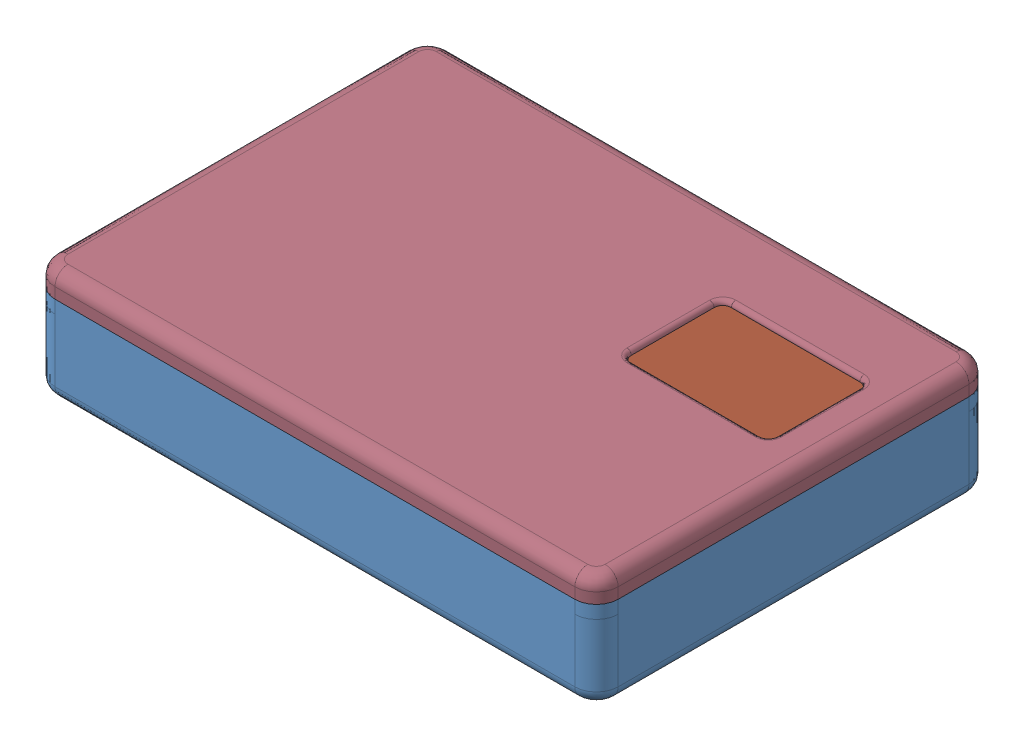
SolidWorks assembly Assembly, configuration Default. Lengths in mm. (continued)
Components (placement in the parent): (continued)
- PCB1_2.step-5: PCB1_2.step [Default] at (-142.0534 45.002 144.8645) x (1 0 -0.000465) z (0 1 0) size (68.54 35.94 11.54) (continued)
  - C21.step-1: C21.step [Default] at origin size (2 1.25 1.4) (continued)
    - Cap_Murata_GRM21BC81C106KA73L_eec.step-1: Cap_Murata_GRM21BC81C106KA73L_eec.step [Default] at (102.7788 62.357 0) x (-1 0 0) z (0 0 1) size (2 1.25 1.4) (continued)
      - 2-41.step-1: 2-41.step [Default] at (0 0 0.01) size (1.98 1.23 1.38)
      - Murata Logo 3.step-1: Murata Logo 3.step [Default] at (-0.1814 -0.5957 1.2901) size (0.53 0.12 0.1)
  - C20.step-1: C20.step [Default] at origin size (2 1.25 1.4)
    - Cap_Murata_GRM21BC81C106KA73L_eec.step-1: Cap_Murata_GRM21BC81C106KA73L_eec.step [Default] at (102.743 59.944 0) x (-1 0 0) z (0 0 1) size (2 1.25 1.4)
      - 1-40.step-1: 1-40.step [Default] at origin size (2 1.25 1.4)
      - 2-41.step-1: 2-41.step [Default] at (0 0 0.01) size (1.98 1.23 1.38)
      - Murata Logo 3.step-1: Murata Logo 3.step [Default] at (-0.1814 -0.5957 1.2901) size (0.53 0.12 0.1)
  - C19.step-1: C19.step [Default] at origin size (0.5 1 0.55)
    - Cap_Murata_GRM1552C1H271GA01J_eec.step-1: Cap_Murata_GRM1552C1H271GA01J_eec.step [Default] at (104.013 57.404 0) x (0 -1 0) z (0 0 1) size (1 0.5 0.55)
      - body-42.step-1: body-42.step [Default] x (-1 0 0) z (0 0 1) size (0.5 0.5 0.55)
      - side-43.step-1: side-43.step [Default] at (-0.2 0.6417 0) x (-1 0 0) z (0 0 1) size (0.25 0.5 0.55)
      - side-43.step-2: side-43.step [Default] at (0.2 0.6417 0.55) x (1 0 0) z (0 0 -1) size (0.25 0.5 0.55)
      - Murata-44.step-1: Murata-44.step [Default] at (-0.859 -0.6449 0.497) size (0.3 0.07 0.02)
  - C18.step-1: C18.step [Default] at origin size (0.8 1.6 0.87)
    - Cap_Wurth_885012206071_eec.step-1: Cap_Wurth_885012206071_eec.step [Default] at (112.903 54.737 0) x (0 -1 0) z (0 0 1) size (1.6 0.8 0.87)
      - terminals.step-1: terminals.step [Default] at origin size (1.6 0.8 0.87)
      - body-45.step-1: body-45.step [Default] at origin size (0.8 0.8 0.87)
      - logo.step-1: logo.step [Default] at (0 0.375 0.87) size (0.36 0.18 0)
  - C17.step-1: C17.step [Default] at origin size (1.25 2 1.4)
    - Cap_Murata_GRM21BC81C106KA73L_eec.step-1: Cap_Murata_GRM21BC81C106KA73L_eec.step [Default] at (90.297 60.071 0) x (0 1 0) z (0 0 1) size (2 1.25 1.4)
      - 1-40.step-1: 1-40.step [Default] at origin size (2 1.25 1.4)
      - 2-41.step-1: 2-41.step [Default] at (0 0 0.01) size (1.98 1.23 1.38)
      - Murata Logo 3.step-1: Murata Logo 3.step [Default] at (-0.1814 -0.5957 1.2901) size (0.53 0.12 0.1)
  - C16.step-1: C16.step [Default] at origin size (1.25 2 1.4)
    - Cap_Murata_GRM21BC81C106KA73L_eec.step-1: Cap_Murata_GRM21BC81C106KA73L_eec.step [Default] at (87.503 60.071 0) x (0 1 0) z (0 0 1) size (2 1.25 1.4)
      - 1-40.step-1: 1-40.step [Default] at origin size (2 1.25 1.4)
      - 2-41.step-1: 2-41.step [Default] at (0 0 0.01) size (1.98 1.23 1.38)
      - Murata Logo 3.step-1: Murata Logo 3.step [Default] at (-0.1814 -0.5957 1.2901) size (0.53 0.12 0.1)
  - C14.step-1: C14.step [Default] at origin size (1.6 0.8 0.87)
    - Cap_Wurth_885012206071_eec.step-1: Cap_Wurth_885012206071_eec.step [Default] at (98.159 54.102 0) x (-1 0 0) z (0 0 1) size (1.6 0.8 0.87)
      - terminals.step-1: terminals.step [Default] at origin size (1.6 0.8 0.87)
      - body-45.step-1: body-45.step [Default] at origin size (0.8 0.8 0.87)
      - logo.step-1: logo.step [Default] at (0 0.375 0.87) size (0.36 0.18 0)
  - C13.step-1: C13.step [Default] at origin size (0.8 1.6 0.87)
    - Cap_Wurth_885012206071_eec.step-1: Cap_Wurth_885012206071_eec.step [Default] at (110.998 54.737 0) x (0 1 0) z (0 0 1) size (1.6 0.8 0.87)
      - terminals.step-1: terminals.step [Default] at origin size (1.6 0.8 0.87)
      - body-45.step-1: body-45.step [Default] at origin size (0.8 0.8 0.87)
      - logo.step-1: logo.step [Default] at (0 0.375 0.87) size (0.36 0.18 0)
  - C12.step-1: C12.step [Default] at origin size (0.8 1.6 0.87)
    - Cap_Wurth_885012206071_eec.step-1: Cap_Wurth_885012206071_eec.step [Default] at (109.22 54.737 0) x (0 1 0) z (0 0 1) size (1.6 0.8 0.87)
      - terminals.step-1: terminals.step [Default] at origin size (1.6 0.8 0.87)
      - body-45.step-1: body-45.step [Default] at origin size (0.8 0.8 0.87)
      - logo.step-1: logo.step [Default] at (0 0.375 0.87) size (0.36 0.18 0)
  - C11.step-1: C11.step [Default] at origin size (2 1.25 1.46)
    - Cap_Murata_GRM21BC71C106KE11L_eec.step-1: Cap_Murata_GRM21BC71C106KE11L_eec.step [Default] at (106.2358 62.357 0) x (-1 0 0) z (0 0 1) size (2 1.25 1.46)
      - body-30.step-1: body-30.step [Default] x (-1 0 0) z (0 0 1) size (1.1 1.25 1.45)
      - side.step-1: side.step [Default] at (-0.7 0.2667 0) x (-1 0 0) z (0 0 1) size (0.45 1.25 1.45)
      - side.step-2: side.step [Default] at (0.7 0.2667 1.45) x (1 0 0) z (0 0 -1) size (0.45 1.25 1.45)
      - Murata.step-1: Murata.step [Default] at (-0.7353 -0.8898 1.447) size (0.61 0.14 0.01)
  - C10.step-1: C10.step [Default] at origin size (2 1.25 1.46)
    - Cap_Murata_GRM21BC71C106KE11L_eec.step-1: Cap_Murata_GRM21BC71C106KE11L_eec.step [Default] at (106.2352 59.944 0) x (-1 0 0) z (0 0 1) size (2 1.25 1.46)
      - body-30.step-1: body-30.step [Default] x (-1 0 0) z (0 0 1) size (1.1 1.25 1.45)
      - side.step-1: side.step [Default] at (-0.7 0.2667 0) x (-1 0 0) z (0 0 1) size (0.45 1.25 1.45)
      - side.step-2: side.step [Default] at (0.7 0.2667 1.45) x (1 0 0) z (0 0 -1) size (0.45 1.25 1.45)
      - Murata.step-1: Murata.step [Default] at (-0.7353 -0.8898 1.447) size (0.61 0.14 0.01)
  - C9.step-1: C9.step [Default] at origin size (0.5 1 0.55)
    - Cap_Murata_GRM1552C1H271GA01J_eec.step-1: Cap_Murata_GRM1552C1H271GA01J_eec.step [Default] at (105.791 57.404 0) x (0 1 0) z (0 0 1) size (1 0.5 0.55)
      - body-42.step-1: body-42.step [Default] x (-1 0 0) z (0 0 1) size (0.5 0.5 0.55)
      - side-43.step-1: side-43.step [Default] at (-0.2 0.6417 0) x (-1 0 0) z (0 0 1) size (0.25 0.5 0.55)
      - side-43.step-2: side-43.step [Default] at (0.2 0.6417 0.55) x (1 0 0) z (0 0 -1) size (0.25 0.5 0.55)
      - Murata-44.step-1: Murata-44.step [Default] at (-0.859 -0.6449 0.497) size (0.3 0.07 0.02)
  - C8.step-1: C8.step [Default] at origin size (0.8 1.6 0.87)
    - Cap_Wurth_885012206071_eec.step-1: Cap_Wurth_885012206071_eec.step [Default] at (118.237 59.309 0) x (0 1 0) z (0 0 1) size (1.6 0.8 0.87)
      - terminals.step-1: terminals.step [Default] at origin size (1.6 0.8 0.87)
      - body-45.step-1: body-45.step [Default] at origin size (0.8 0.8 0.87)
      - logo.step-1: logo.step [Default] at (0 0.375 0.87) size (0.36 0.18 0)
  - C7.step-1: C7.step [Default] at origin size (0.8 1.6 0.87)
    - Cap_Wurth_885012206071_eec.step-1: Cap_Wurth_885012206071_eec.step [Default] at (109.728 59.182 0) x (0 1 0) z (0 0 1) size (1.6 0.8 0.87)
      - terminals.step-1: terminals.step [Default] at origin size (1.6 0.8 0.87)
      - body-45.step-1: body-45.step [Default] at origin size (0.8 0.8 0.87)
      - logo.step-1: logo.step [Default] at (0 0.375 0.87) size (0.36 0.18 0)
  - C6.step-1: C6.step [Default] at origin size (0.9 1.7 0.9)
    - 6262525248.step-1: 6262525248.step [Default] at (74.295 49.53 -1.3104) size (0.9 1 0.9)
      - Extruded-46.step-1: Extruded-46.step [Default] at origin size (0.9 1 0.9)
    - 6262525088.step-1: 6262525088.step [Default] at (74.295 48.855 -1.3104) size (0.9 0.35 0.9)
      - Extruded-47.step-1: Extruded-47.step [Default] at origin size (0.9 0.35 0.9)
    - 6262525088.step-2: 6262525088.step [Default] at (74.295 50.205 -1.3104) size (0.9 0.35 0.9)
      - Extruded-47.step-1: Extruded-47.step [Default] at origin size (0.9 0.35 0.9)
  - C5.step-1: C5.step [Default] at origin size (0.9 1.7 0.9)
    - 6262525248.step-1: 6262525248.step [Default] at (74.295 52.959 -1.3104) size (0.9 1 0.9)
      - Extruded-46.step-1: Extruded-46.step [Default] at origin size (0.9 1 0.9)
    - 6262525088.step-1: 6262525088.step [Default] at (74.295 53.634 -1.3104) size (0.9 0.35 0.9)
      - Extruded-47.step-1: Extruded-47.step [Default] at origin size (0.9 0.35 0.9)
    - 6262525088.step-2: 6262525088.step [Default] at (74.295 52.284 -1.3104) size (0.9 0.35 0.9)
      - Extruded-47.step-1: Extruded-47.step [Default] at origin size (0.9 0.35 0.9)
  - C4.step-1: C4.step [Default] at origin size (1.25 2 1.45)
    - 6259391984.step-1: 6259391984.step [Default] at (85.471 49.217 0) x (0 -1 0) z (0 0 1) size (2 1.25 1.45)
      - Fillet1-48.step-1: Fillet1-48.step [Default] at origin size (0.45 1.25 1.45)
      - Fillet2-49.step-1: Fillet2-49.step [Default] at origin size (0.45 1.25 1.45)
      - body2-50.step-1: body2-50.step [Default] at origin size (1.1 1.22 1.42)
  - C3.step-1: C3.step [Default] at origin size (2 1.25 1.4)
    - Cap_Murata_GRM21BC81C106KA73L_eec.step-1: Cap_Murata_GRM21BC81C106KA73L_eec.step [Default] at (124.46 53.594 0) size (2 1.25 1.4)
      - 1-40.step-1: 1-40.step [Default] at origin size (2 1.25 1.4)
      - 2-41.step-1: 2-41.step [Default] at (0 0 0.01) size (1.98 1.23 1.38)
      - Murata Logo 3.step-1: Murata Logo 3.step [Default] at (-0.1814 -0.5957 1.2901) size (0.53 0.12 0.1)
  - C2.step-1: C2.step [Default] at origin size (1.25 2 1.4)
    - Cap_Murata_GRM21BC81C106KA73L_eec.step-1: Cap_Murata_GRM21BC81C106KA73L_eec.step [Default] at (121.285 53.213 0) x (0 1 0) z (0 0 1) size (2 1.25 1.4)
      - 1-40.step-1: 1-40.step [Default] at origin size (2 1.25 1.4)
      - 2-41.step-1: 2-41.step [Default] at (0 0 0.01) size (1.98 1.23 1.38)
      - Murata Logo 3.step-1: Murata Logo 3.step [Default] at (-0.1814 -0.5957 1.2901) size (0.53 0.12 0.1)
  - C1.step-1: C1.step [Default] at origin size (1.6 0.8 0.8)
    - 6259394864.step-1: 6259394864.step [Default] at (124.46 44.577 0.4) x (0 -1 0) z (-1 0 0) size (0.8 0.8 1.6)
- 18650 battery holder-1: 18650 battery holder [Výchozí] at (48.1858 46.5359 152.1637) x (0 0 1) z (-1 0 0) size (39.8 18.9 86.4)
  - 18650 baterie-1: 18650 baterie [Výchozí] at (-5.3689 1.7057 32.3879) size (18.5 18.5 64.78)
  - 18650 holder 2x-1: 18650 holder 2x [Výchozí] at (-14.7189 1.7057 25.8879) size (39.8 15.3 86.4)
  - 18650 baterie-2: 18650 baterie [Výchozí] at (-24.0689 1.7057 32.3879) size (18.5 18.5 64.78)
- ASSEMBLY_AP214.STEP-1: ASSEMBLY_AP214.STEP [Default] at (-14.6491 31.0882 66.6987) x (1 0 -0.000465) z (0.000465 0 1) size (17.79 12.75 33.03)
  - Crystal_Low_Profile.STEP-1: Crystal_Low_Profile.STEP [Default] at (9.717 16.7052 22.6754) x (0 0 -1) z (0 1 0) size (3.81 1.63 0.79)
    - Fusion001.STEP-1: Fusion001.STEP [Default] at origin size (3.81 1.63 0.79)
  - board.STEP-1: board.STEP [Default] at (5.4752 15.0552 41.6975) size (17.78 1.67 33.02)
  - ATmega.STEP-1: ATmega.STEP [Default] at (14.3652 16.8027 27.7275) x (0.707107 0 0.707107) z (-0.707107 0 0.707107) size (9 1.1 9)
  - cap_603.STEP-1: cap_603.STEP [Default] at (10.3417 16.7052 40.4401) x (0 0 -1) z (1 0 0) size (1.6 0.8 0.8)
  - cap_603.STEP-2: cap_603.STEP [Default] at (13.6922 16.7052 34.8585) size (1.6 0.8 0.8)
  - cap_603.STEP-3: cap_603.STEP [Default] at (11.8634 16.7052 21.6759) size (1.6 0.8 0.8)
  - cap_603.STEP-4: cap_603.STEP [Default] at (17.4768 16.7052 12.8875) size (1.6 0.8 0.8)
  - res_603.STEP-1: res_603.STEP [Default] at (10.4218 16.7052 37.2651) x (0 0 -1) z (1 0 0) size (1.6 0.5 0.8)
  - res_603.STEP-2: res_603.STEP [Default] at (19.5912 16.7052 37.5953) x (0 0 -1) z (1 0 0) size (1.6 0.5 0.8)
  - res_603.STEP-3: res_603.STEP [Default] at (15.1652 16.7052 14.6275) x (-1 0 0) z (0 0 -1) size (1.6 0.5 0.8)
  - condensateurTantale_106C_D_faut.STEP-1: condensateurTantale_106C_D_faut.STEP [Default] at (10.1742 17.5052 15.6625) x (0 0 -1) z (1 0 0) size (3.2 1.6 1.6)
  - condensateurTantale_106C_D_faut.STEP-2: condensateurTantale_106C_D_faut.STEP [Default] at (18.6832 17.5052 17.5675) x (0 0 -1) z (1 0 0) size (3.2 1.6 1.6)
  - SOT23-5.STEP-1: SOT23-5.STEP [Default] at (14.3653 16.6848 17.5167) x (1 0 0) z (0 1 0) size (2.84 3 1.19)
  - Surface Mount Chip LED 3.2x1.6mm.STEP-1: Surface Mount Chip LED 3.2x1.6mm.STEP [Default] at (18.7112 16.7112 39.0103) x (0 0 1) z (0 1 0) size (1.92 0.96 0.79)
  - Surface Mount Chip LED 3.2x1.6mm.STEP-2: Surface Mount Chip LED 3.2x1.6mm.STEP [Default] at (13.4306 16.7112 20.3081) x (1 0 0) z (0 1 0) size (1.92 0.96 0.79)
  - TACTILE-SWITCH-SMD-ALT01.STEP-1: TACTILE-SWITCH-SMD-ALT01.STEP [Default] at (14.4922 16.7052 39.0305) size (6.4 1.4 5.22)
  - Pin Header 1x12 TH Pitch 2.54mm.STEP-1: Pin Header 1x12 TH Pitch 2.54mm.STEP [Default] at (6.7452 15.0555 40.428) x (0 0.000074 -1) z (0 -1 -0.000074) size (30.49 2.55 12.71)
  - Pin Header 1x12 TH Pitch 2.54mm.STEP-2: Pin Header 1x12 TH Pitch 2.54mm.STEP [Default] at (21.9852 15.0555 40.428) x (0 0.000074 -1) z (0 -1 -0.000074) size (30.49 2.55 12.71)
  - Pin Header 1x2 TH Pitch 2.54mm.STEP-1: Pin Header 1x2 TH Pitch 2.54mm.STEP [Default] at (19.0642 15.0566 31.6645) x (0 0 1) z (0 -1 0) size (5.09 2.55 12.71)
  - Pin Header 1x2 TH Pitch 2.54mm.STEP-2: Pin Header 1x2 TH Pitch 2.54mm.STEP [Default] at (19.0642 15.0565 21.2505) x (0 0.000074 1) z (0 -1 0.000074) size (5.09 2.55 12.71)
  - Pin Header 1x6 TH Pitch 2.54mm.STEP-1: Pin Header 1x6 TH Pitch 2.54mm.STEP [Default] at (8.0152 15.0566 9.9475) x (1 0 0) z (0 -1 0) size (15.25 2.55 12.71)
  - solder.STEP-1: solder.STEP [Default] at (6.7452 16.7152 40.4275) size (1.8 1.45 1.8)
  - solder.STEP-2: solder.STEP [Default] at (21.9852 16.7152 40.4275) size (1.8 1.45 1.8)
  - solder.STEP-3: solder.STEP [Default] at (19.0642 16.7152 23.7905) size (1.8 1.45 1.8)
  - solder.STEP-4: solder.STEP [Default] at (19.0642 16.7152 34.2045) size (1.8 1.45 1.8)
  - solder.STEP-5: solder.STEP [Default] at (20.7152 16.7152 9.9475) size (1.8 1.45 1.8)
  - solder.STEP-6: solder.STEP [Default] at (6.7452 16.7152 37.8875) size (1.8 1.45 1.8)
  - solder.STEP-7: solder.STEP [Default] at (6.7452 16.7152 35.3475) size (1.8 1.45 1.8)
  - solder.STEP-8: solder.STEP [Default] at (6.7452 16.7152 32.8075) size (1.8 1.45 1.8)
  - solder.STEP-9: solder.STEP [Default] at (6.7452 16.7152 30.2675) size (1.8 1.45 1.8)
  - solder.STEP-10: solder.STEP [Default] at (6.7452 16.7152 27.7275) size (1.8 1.45 1.8)
  - solder.STEP-11: solder.STEP [Default] at (6.7452 16.7152 25.1875) size (1.8 1.45 1.8)
  - solder.STEP-12: solder.STEP [Default] at (6.7452 16.7152 22.6475) size (1.8 1.45 1.8)
  - solder.STEP-13: solder.STEP [Default] at (6.7452 16.7152 20.1075) size (1.8 1.45 1.8)
  - solder.STEP-14: solder.STEP [Default] at (6.7452 16.7152 17.5675) size (1.8 1.45 1.8)
  - solder.STEP-15: solder.STEP [Default] at (6.7452 16.7152 15.0275) size (1.8 1.45 1.8)
  - solder.STEP-16: solder.STEP [Default] at (6.7452 16.7152 12.4875) size (1.8 1.45 1.8)
  - solder.STEP-17: solder.STEP [Default] at (21.9852 16.7152 37.8875) size (1.8 1.45 1.8)
  - solder.STEP-18: solder.STEP [Default] at (21.9852 16.7152 35.3475) size (1.8 1.45 1.8)
  - solder.STEP-19: solder.STEP [Default] at (21.9852 16.7152 32.8075) size (1.8 1.45 1.8)
  - solder.STEP-20: solder.STEP [Default] at (21.9852 16.7152 30.2675) size (1.8 1.45 1.8)
  - solder.STEP-21: solder.STEP [Default] at (21.9852 16.7152 27.7275) size (1.8 1.45 1.8)
  - solder.STEP-22: solder.STEP [Default] at (21.9852 16.7152 25.1875) size (1.8 1.45 1.8)
  - solder.STEP-23: solder.STEP [Default] at (21.9852 16.7152 22.6475) size (1.8 1.45 1.8)
  - solder.STEP-24: solder.STEP [Default] at (21.9852 16.7152 20.1075) size (1.8 1.45 1.8)
  - solder.STEP-25: solder.STEP [Default] at (21.9852 16.7152 17.5675) size (1.8 1.45 1.8)
  - solder.STEP-26: solder.STEP [Default] at (21.9852 16.7152 15.0275) size (1.8 1.45 1.8)
  - solder.STEP-27: solder.STEP [Default] at (21.9852 16.7152 12.4875) size (1.8 1.45 1.8)
  - solder.STEP-28: solder.STEP [Default] at (19.0642 16.7152 21.2505) size (1.8 1.45 1.8)
  - solder.STEP-29: solder.STEP [Default] at (19.0642 16.7152 31.6645) size (1.8 1.45 1.8)
  - solder.STEP-30: solder.STEP [Default] at (18.1752 16.7152 9.9475) size (1.8 1.45 1.8)
  - solder.STEP-31: solder.STEP [Default] at (15.6352 16.7152 9.9475) size (1.8 1.45 1.8)
  - solder.STEP-32: solder.STEP [Default] at (13.0952 16.7152 9.9475) size (1.8 1.45 1.8)
  - solder.STEP-33: solder.STEP [Default] at (10.5552 16.7152 9.9475) size (1.8 1.45 1.8)
  - solder.STEP-34: solder.STEP [Default] at (8.0152 16.7152 9.9475) size (1.8 1.45 1.8)
- OLED+pines-1: OLED+pines [Predeterminado] at (21.6975 58.3828 63.8912) x (1 0 0.000181) z (-0.000181 0 1) size (35.65 11.1 33.6)
  - oled-1: oled [Default] at (4.7217 0.2089 48.7) size (35.65 2.6 33.6)
  - pin - copia-1: pin - copia [Predeterminado] at (1.2367 3.2089 21.125) x (-1 0 0) z (0 0 1) size (2.54 11.1 2.4)
  - pin - copia-2: pin - copia [Predeterminado] at (3.7767 3.2089 21.125) x (-1 0 0) z (0 0 1) size (2.54 11.1 2.4)
  - pin - copia-3: pin - copia [Predeterminado] at (6.3167 3.2089 21.125) x (-1 0 0) z (0 0 1) size (2.54 11.1 2.4)
  - pin - copia-4: pin - copia [Predeterminado] at (8.8567 3.2089 21.125) x (-1 0 0) z (0 0 1) size (2.54 11.1 2.4)
- Part2-1: Part2 [Default] at (-77.6648 62.0917 159.8448) x (1 0 0) z (0 -1 0) size (130 91 20.5)
- tact switch SMD IT-1187A (5x5x4.3) smd T209.step-1: tact switch SMD IT-1187A (5x5x4.3) smd T209.step [Default] at (-0.2757 52.1999 72.8448) x (1 0 0) z (0 1 0) size (6.4 4.3 5.2)
- pan cross head_am-1: pan cross head_am [B18.6.7M - M2 x 0.4 x 2.5 Type I Cross Recessed PHMS --2.5N] at (11.1952 61.5744 85.3448) x (0 -1 0) z (0.41189 0 0.911234) size (4.08 4 4)
- pan cross head_am-3: pan cross head_am [B18.6.7M - M2 x 0.4 x 2.5 Type I Cross Recessed PHMS --2.5N] at (11.1952 61.2627 113.7448) x (0 -1 0) z (0 0 1) size (4.08 4 4)
- pan cross head_am-4: pan cross head_am [B18.6.7M - M2 x 0.4 x 2.5 Type I Cross Recessed PHMS --2.5N] at (41.6352 61.5855 113.7448) x (0 -1 0) z (0.003702 0 0.999993) size (4.08 4 4)
- pan cross head_am-5: pan cross head_am [B18.6.7M - M2 x 0.4 x 2.5 Type I Cross Recessed PHMS --2.5N] at (41.6352 61.4182 85.3448) x (0 -1 0) z (-0.200508 0 0.979692) size (4.08 4 4)
- pan cross head_am-6: pan cross head_am [B18.6.7M - M3 x 0.5 x 5 Type I Cross Recessed PHMS --5N] at (-67.5348 47.4039 79.4248) x (0 -1 0) z (0.029786 0 0.999556) size (7.37 5.6 5.6)
- pan cross head_am-7: pan cross head_am [B18.6.7M - M3 x 0.5 x 6 Type I Cross Recessed PHMS --6N] at (-67.5348 47.3904 106.6048) x (0 -1 0) z (0.378981 0 0.925404) size (8.37 5.6 5.6)
- pan cross head_am-8: pan cross head_am [B18.6.7M - M3 x 0.5 x 6 Type I Cross Recessed PHMS --6N] at (-13.2948 47.3877 79.4248) x (0 -1 0) z (0.060232 0 0.998184) size (8.37 5.6 5.6)
- pan cross head_am-9: pan cross head_am [B18.6.7M - M3 x 0.5 x 6 Type I Cross Recessed PHMS --6N] at (-13.2948 47.4047 106.6048) x (0 -1 0) z (0.088664 0 0.996062) size (8.37 5.6 5.6)
Mates (geometry in assembly coordinates):
- Concentric2: concentric aligned: circle of Part1-1; circle of PCB1_2.step-5/Board.step-1/Open CASCADE STEP translator 7.5 1.1.1.step-1
- Coincident5: coincident aligned: plane of Part1-1 through (-67.5348 44.5917 106.6048) normal (0 1 0); circle of PCB1_2.step-5/Board.step-1/Open CASCADE STEP translator 7.5 1.1.1.step-1
- Coincident6: coincident aligned: plane of Part1-1 through (-13.2948 44.5917 106.6048) normal (0 1 0); circle of PCB1_2.step-5/Board.step-1/Open CASCADE STEP translator 7.5 1.1.1.step-1
- Coincident7: coincident aligned: plane of Part1-1 through (-13.2948 44.5917 79.4248) normal (0 1 0); circle of PCB1_2.step-5/Board.step-1/Open CASCADE STEP translator 7.5 1.1.1.step-1
- Coincident8: coincident anti-aligned: plane of Part1-1 through (-77.6648 38.5917 68.8448) normal (0 1 0); plane of 18650 battery holder-1/18650 holder 2x-1 through (18.4979 38.5917 137.4448) normal (0 -1 0)
- Coincident10: coincident: plane of Part1-1 through (-77.6648 53.5917 157.3448) normal (0 0 -1); line of 18650 battery holder-1/18650 holder 2x-1 through (-3.0521 45.5917 157.3448) axis (-1 0 0)
- Parallel3: parallel anti-aligned: plane of PCB1_2.step-5/Board.step-1/Open CASCADE STEP translator 7.5 1.1.1.step-1 through (-9.2272 44.5917 110.8937) normal (1 0 -0.000465); plane of ASSEMBLY_AP214.STEP-1/board.STEP-1 through (-9.1545 47.7934 108.3937) normal (-1 0 0.000465)
- Concentric7: concentric anti-aligned: circle of Part1-1; circle of OLED+pines-1/oled-1
- Coincident12: coincident anti-aligned: plane of Part1-1 through (41.6352 58.5917 113.7448) normal (0 1 0); plane of OLED+pines-1/oled-1 through (26.4104 58.5917 112.5921) normal (0 -1 0)
- Coincident14: coincident anti-aligned: plane of Part1-1 through (41.6352 58.5917 85.3448) normal (0 1 0); plane of OLED+pines-1/oled-1 through (26.4104 58.5917 112.5921) normal (0 -1 0)
- Coincident15: coincident anti-aligned: plane of Part1-1 through (-77.6648 53.5917 71.3448) normal (0 0 1); circle of tact switch SMD IT-1187A (5x5x4.3) smd T209.step-1
- Parallel4: parallel anti-aligned: line of Part1-1 through (47.3352 56.5917 68.8448) axis (-1 0 0); line of Part2-1 through (-72.6648 59.0917 68.8448) axis (1 0 0)
- Concentric12: concentric aligned: cylinder of Part1-1 through (11.1952 52.5917 85.3448) axis (0 1 0) radius 1.5; cylinder of pan cross head_am-1 through (11.1952 86.9744 85.3448) axis (0 1 0) radius 1
- Concentric13: concentric aligned: cylinder of Part1-1 through (11.1952 52.5917 113.7448) axis (0 1 0) radius 1.5; cylinder of pan cross head_am-3 through (11.1952 86.6627 113.7448) axis (0 1 0) radius 1
- Concentric14: concentric aligned: cylinder of Part1-1 through (41.6352 52.5917 113.7448) axis (0 1 0) radius 1.5; cylinder of pan cross head_am-4 through (41.6352 86.9855 113.7448) axis (0 1 0) radius 1
- Concentric17: concentric aligned: cylinder of Part1-1 through (41.6352 52.5917 85.3448) axis (0 1 0) radius 1.5; cylinder of pan cross head_am-5 through (41.6352 86.8182 85.3448) axis (0 1 0) radius 1
- Concentric19: concentric aligned: cylinder of Part1-1 through (-67.5348 39.5917 79.4248) axis (0 1 0) radius 1.5; cylinder of pan cross head_am-6 through (-67.5348 72.8039 79.4248) axis (0 1 0) radius 1.5
- Concentric20: concentric aligned: cylinder of Part1-1 through (-67.5348 39.5917 106.6048) axis (0 1 0) radius 1.5; cylinder of pan cross head_am-7 through (-67.5348 72.7904 106.6048) axis (0 1 0) radius 1.5
- Concentric21: concentric aligned: cylinder of Part1-1 through (-13.2948 39.5917 79.4248) axis (0 1 0) radius 1.5; cylinder of pan cross head_am-8 through (-13.2948 72.7877 79.4248) axis (0 1 0) radius 1.5
- Concentric22: concentric aligned: cylinder of Part1-1 through (-13.2948 39.5917 106.6048) axis (0 1 0) radius 1.5; cylinder of pan cross head_am-9 through (-13.2948 72.8047 106.6048) axis (0 1 0) radius 1.5
- Concentric24: concentric aligned: cylinder of Part1-1 through (-1.1648 40.5917 113.3448) axis (0 1 0) radius 1.5; cylinder of Part2-1 through (-1.1648 41.5917 113.3448) axis (0 1 0) radius 1.4
- Coincident21: coincident anti-aligned: plane of Part1-1 through (-77.6648 56.5917 68.8448) normal (0 1 0); plane of Part2-1 through (-77.6648 56.5917 159.8448) normal (0 -1 0)
